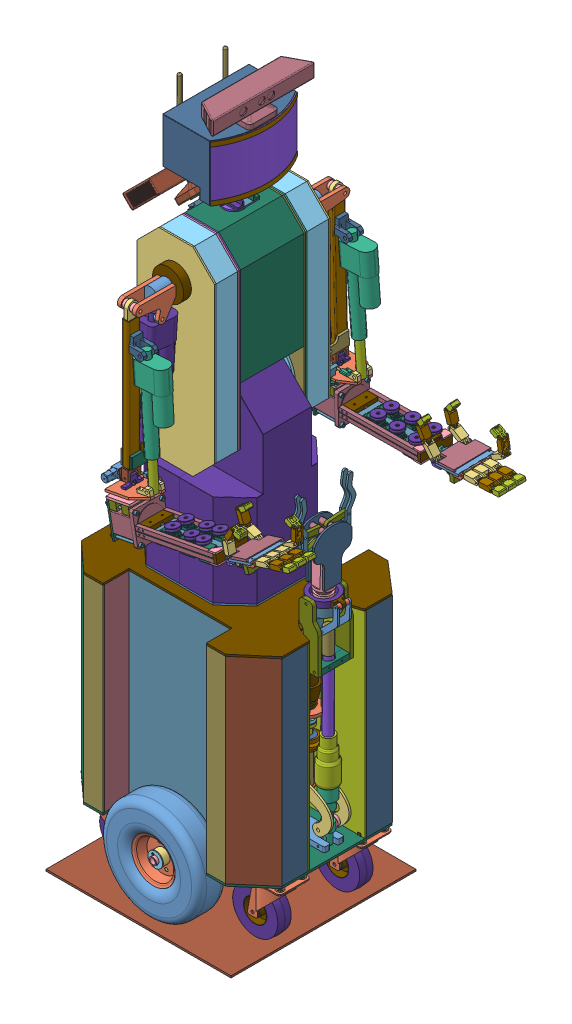
SolidWorks assembly sorbot, configuration По умолчанию. Lengths in mm. (continued)
Components (placement in the parent): (continued)
- arm.drive.p2-1: arm.drive.p2 [По умолчанию] at (43.6014 1241.2974 -35.5806) x (-0.089772 0 -0.995962) z (0.995962 0 -0.089772) size (134 5 24)
- arm.drive.p3-1: arm.drive.p3 [По умолчанию] at (3.7745 1243.7974 -50.7442) x (0 0 -1) z (0.174973 -0.984573 0) size (133.1 20 20)
- body.frame.p1-left-1: body.frame.p1-left [По умолчанию] at (-12.5682 795.4677 -226.3595) x (1 0 0) z (0 0 1) size (210 537.56 4)
- arm.drive.motor-1: arm.drive.motor [По умолчанию] at (-94.8762 1249.003 -67.2442) x (-0.533544 -0.845772 0) z (0.845772 -0.533544 0) size (117 39.5 152)
- arm.drive.motor.pair-1: arm.drive.motor.pair [По умолчанию] at (-76.8976 1162.9951 -205.8595) x (-0.885964 0.463755 0) z (0.463755 0.885964 0) size (117 39.5 152)
- arm.actuator.p2-5: arm.actuator.p2 [Default] at (-12.384 1125.8641 -368.5595) x (-0.005174 -0.093519 0.995604) z (0.999986 0 0.005196) size (20 180 20)
- arm.drive.p5-1: arm.drive.p5 [По умолчанию] at (3.7745 1243.7974 -58.7442) x (1 0 0) z (0 -1 0) size (34 8 34)
- arm.drive.p6-1: arm.drive.p6 [По умолчанию] at (3.7745 1243.7974 -50.7442) x (1 0 0) z (0 1 0) size (40 12 40)
- arm.drive.p3-2: arm.drive.p3 [По умолчанию] at (-20.8275 1162.0905 -222.3595) x (0 0 1) z (-0.923728 -0.383049 0) size (133.1 20 20)
- arm.drive.p5-2: arm.drive.p5 [По умолчанию] at (-20.8275 1162.0905 -214.3595) x (1 0 0) z (0 1 0) size (34 8 34)
- arm.drive.p6-2: arm.drive.p6 [По умолчанию] at (-20.8275 1162.0905 -222.3595) x (1 0.000029 0) z (0.000029 -1 0) size (40 12 40)
- arm.drive.p2-pair-1: arm.drive.p2-pair [По умолчанию] at (50.3811 1159.5904 -236.7848) x (-0.315418 0 0.948953) z (-0.948953 0 -0.315418) size (144 5 24)
- m14.nut-1: m14.nut [По умолчанию] at (-20.8275 1162.0905 -118.4852) x (0.513607 -0.858026 0) z (0.858026 0.513607 0) size (25.4 10.5 22.2)
- arm.drive.p7-2: arm.drive.p7 [По умолчанию] at (-14.5918 1147.0905 -123.4852) x (0 0 1) z (-1 0 0) size (28 15 59.47)
- arm.drive.p7-3: arm.drive.p7 [По умолчанию] at (-14.5918 1177.0905 -123.4852) x (0 0 -1) z (-1 0 0) size (28 15 59.47)
- arm.drive.p7-4: arm.drive.p7 [По умолчанию] at (10.1478 1228.9206 -145.3) x (0 0 1) z (-1 0 0) size (28 15 59.47)
- arm.drive.p7-5: arm.drive.p7 [По умолчанию] at (10.1478 1258.9206 -145.3) x (0 0 -1) z (-1 0 0) size (28 15 59.47)
- m14.nut-2: m14.nut [По умолчанию] at (3.7745 1243.7974 -150.3) x (-0.999875 0.015784 0) z (0.015784 0.999875 0) size (25.4 10.5 22.2)
- arm.drive.p1.m1-1: arm.drive.p1.m1 [По умолчанию] at (28.6519 1164.5905 -225.3595) x (0 1 0) z (-1 0 0) size (10 12 40)
- arm.drive.p1.m1-2: arm.drive.p1.m1 [По умолчанию] at (28.6519 1149.5905 -225.3595) x (0 1 0) z (-1 0 0) size (10 12 40)
- body.frame.p4.external-1: body.frame.p4.external [По умолчанию] at (-12.7111 795.3889 -292.3595) x (1 -0.000113 0) z (0 0 1) size (210 537.56 4)
- body.frame.p4.external-2: body.frame.p4.external [По умолчанию] at (-12.8242 795.3889 15.2558) x (1 -0.000113 0) z (0 0 1) size (210 537.56 4)
- arm.drive.p1.m1-3: arm.drive.p1.m1 [По умолчанию] at (65.4163 1231.2974 -47.7442) x (0 1 0) z (1 0 0) size (10 12 40)
- arm.drive.p1.m1-4: arm.drive.p1.m1 [По умолчанию] at (65.4163 1246.2974 -47.7442) x (0 1 0) z (1 0 0) size (10 12 40)
- body.frame.p4.right-1: body.frame.p4.right [По умолчанию] at (-12.4903 795.5195 -46.7442) x (1 0 0) z (0 0 1) size (210 537.56 4)
- arm.drive.p8-1: arm.drive.p8 [По умолчанию] at (-20.8275 1162.0905 -72.7442) x (-0.999995 0.003205 0) z (-0.003205 -0.999995 0) size (24 35.5 24)
- arm.drive.p8-2: arm.drive.p8 [По умолчанию] at (3.7745 1243.7974 -200.3595) x (1 0 0) z (0 -1 0) size (24 35.5 24)
- man1.drive1-1: man1.drive1 [По умолчанию] at (-119.3768 640.728 -141.6211) x (0.999934 0 -0.01146) z (0 1 0) size (50 50 148.25)
- body.tilit.planetary.drive.fixture.p1-1: body.tilit.planetary.drive.fixture.p1 [По умолчанию] at (-119.3768 612.7934 -141.6211) size (85 10 85)
- body.tilit.planetary.drive.fixture.p2-1: body.tilit.planetary.drive.fixture.p2 [По умолчанию] at (-119.3768 622.7934 -141.6211) size (85 4 85)
- tilt.thread.rod.fixture.2-2: tilt.thread.rod.fixture.2 [По умолчанию] at (-119.3768 793.5591 -141.6211) x (-0.837169 0 -0.546944) z (-0.546944 0 0.837169) size (40 26 40)
- body.tilit.planetary.drive.fixture.p3-1: body.tilit.planetary.drive.fixture.p3 [По умолчанию] at (-119.3768 695.728 -141.6211) size (68 8 68)
- body.tilit.planetary.drive.fixture.p4-1: body.tilit.planetary.drive.fixture.p4 [По умолчанию] at (-119.3768 753.9526 -141.6211) x (0.997546 0 -0.070011) z (0.070011 0 0.997546) size (70 9 70)
- body.tilit.planetary.drive.fixture.p5-1: body.tilit.planetary.drive.fixture.p5 [По умолчанию] at (-148.8664 612.7934 -141.6211) size (5 157 5)
- m6.nut-13: m6.nut [По умолчанию] at (-148.8664 613.2934 -141.6211) size (10 5.5 11.55)
- body.tilit.planetary.drive.fixture.p5-2: body.tilit.planetary.drive.fixture.p5 [По умолчанию] at (-89.8872 612.7934 -141.6211) size (5 157 5)
- body.tilit.planetary.drive.fixture.p5-3: body.tilit.planetary.drive.fixture.p5 [По умолчанию] at (-119.3768 612.7934 -112.1315) size (5 157 5)
- body.tilit.planetary.drive.fixture.p5-4: body.tilit.planetary.drive.fixture.p5 [По умолчанию] at (-119.3768 612.7934 -171.1107) size (5 157 5)
- m6.nut-14: m6.nut [По умолчанию] at (-89.8872 613.2934 -141.6211) size (10 5.5 11.55)
- m6.nut-15: m6.nut [По умолчанию] at (-119.3768 613.2934 -171.1107) x (0.598875 0 -0.800843) z (0.800843 0 0.598875) size (10 5.5 11.55)
- m6.nut-16: m6.nut [По умолчанию] at (-119.3768 613.2934 -112.1315) x (-0.286054 0 -0.958214) z (0.958214 0 -0.286054) size (10 5.5 11.55)
- m6.nut-17: m6.nut [По умолчанию] at (-119.3768 768.4526 -112.1315) x (-0.837169 0 -0.546944) z (-0.546944 0 0.837169) size (10 5.5 11.55)
- m6.nut-18: m6.nut [По умолчанию] at (-89.8872 768.4526 -141.6211) x (-0.837169 0 -0.546944) z (-0.546944 0 0.837169) size (10 5.5 11.55)
- m6.nut-19: m6.nut [По умолчанию] at (-119.3768 768.4526 -171.1107) x (-0.837169 0 -0.546944) z (-0.546944 0 0.837169) size (10 5.5 11.55)
- m6.nut-20: m6.nut [По умолчанию] at (-148.8664 768.4526 -141.6211) x (-0.837169 0 -0.546944) z (-0.546944 0 0.837169) size (10 5.5 11.55)
- m6.nut-21: m6.nut [По умолчанию] at (-29.5996 1324.99 9.9014) x (-0.526603 0.850111 0) z (0 0 1) size (10 5.5 11.55)
- m6.6.50mm-1: m6.6.50mm [По умолчанию] at (4.3029 1345.9909 9.9014) x (0.525089 -0.847668 0.075763) z (-0.039897 0.064407 0.997126) size (10 56 10)
- m4.nut-1: m4.nut [По умолчанию] at (-35.3987 1340.8364 4.6679) x (1 0 0) z (0 -1 0) size (6.86 5 7.92)
- m4.nut-2: m4.nut [По умолчанию] at (-103.2224 997.8992 -35.7442) x (1 0 0) z (0 -1 0) size (6.86 5 7.92)
- arm.rotate-1: arm.rotate [По умолчанию] at (22.4782 854.2475 144.4763) x (0 0 1) z (-0.185706 0.982605 0) size (85.26 111.5 91.5)
  - SY85STH65-2808A-1: SY85STH65-2808A [По умолчанию] at (-4.2017 8.56 0) size (85.26 96.5 85)
  - m6.6.80mm-1: m6.6.80mm [По умолчанию] at (-39.0017 18.56 -34.8) size (10 86 10)
  - m6.6.80mm-2: m6.6.80mm [По умолчанию] at (30.5983 18.56 34.8) size (10 86 10)
  - m6.6.80mm-3: m6.6.80mm [По умолчанию] at (30.5983 18.56 -34.8) size (10 86 10)
  - m6.6.80mm-4: m6.6.80mm [По умолчанию] at (-39.0017 18.56 34.8) size (10 86 10)
  - arm.rotate.p2-2: arm.rotate.p2 [По умолчанию] at (-46.7017 -46.44 42.5) x (1 0 0) z (0 -1 0) size (85 91.5 5)
  - m6.nut-1: m6.nut [По умолчанию] at (30.5983 -56.94 34.8) size (10 5.5 11.55)
  - m6.nut-2: m6.nut [По умолчанию] at (-39.0017 -56.94 -34.8) size (10 5.5 11.55)
  - m6.nut-3: m6.nut [По умолчанию] at (-39.0017 -56.94 34.8) size (10 5.5 11.55)
  - m6.nut-4: m6.nut [По умолчанию] at (30.5983 -56.94 -34.8) size (10 5.5 11.55)
  - arm.rotate.p1-2: arm.rotate.p1 [По умолчанию] at (-4.2017 8.56 38) x (1 0 0) z (0 -1 0) size (85 21 20)
  - arm.rotate.p1-3: arm.rotate.p1 [По умолчанию] at (-4.2017 -26.44 38) x (1 0 0) z (0 -1 0) size (85 21 20)
- arm.rotate.p8-1: arm.rotate.p8 [По умолчанию] at (-48.9081 912.5039 130.5417) x (-0.185706 0.982605 0) z (0 0 1) size (25 12 48)
- arm.rotate.p9-1: arm.rotate.p9 [По умолчанию] at (42.4949 859.0482 172.7746) x (0.982605 0.185706 0) z (0 0 1) size (30 10 65)
- arm.rotate.p9-2: arm.rotate.p9 [По умолчанию] at (72.3444 862.6542 172.7746) x (-0.982605 -0.185706 0) z (0 0 1) size (30 10 65)
- arm.elbow.rotate.p1-1: arm.elbow.rotate.p1 [По умолчанию] at (-55.7977 924.3811 168.7746) x (-0.185706 0.982605 0) z (0 0 -1) size (21.9 27.89 71.5)
- arm.rotate.p6-1: arm.rotate.p6 [По умолчанию] at (20.223 919.4631 140.2746) x (0 0 1) z (-0.982605 -0.185706 0) size (85 6 102)
- arm.rotate.p7-1: arm.rotate.p7 [По умолчанию] at (81.3033 937.1131 170.2746) x (-0.185706 0.982605 0) z (0 0 -1) size (16 36 10)
- arm.rotate.p7-2: arm.rotate.p7 [По умолчанию] at (81.3033 937.1131 140.2746) x (-0.185706 0.982605 0) z (0 0 -1) size (16 36 10)
- arm.rotate.p10-1: arm.rotate.p10 [По умолчанию] at (-37.1666 892.8424 182.7746) x (0 0 -1) z (0.982605 0.185706 0) size (85 6 65)
- arm.elbow.rotate.bearing-1: arm.elbow.rotate.bearing [По умолчанию] at (-7.5173 911.1932 140.056) x (-0.183128 -0.03461 0.98248) z (-0.96539 -0.182453 -0.18637) size (61.4 10 61.4)
  - arm.elbow.rotate.bearing.p1-1: arm.elbow.rotate.bearing.p1 [По умолчанию] at (0.2225 -3.7755 0) size (61.4 4.5 61.4)
  - ball.10mm-1: ball.10mm [По умолчанию] at (0.0947 -1.5255 -24.7664) size (10 10 10)
  - ball.10mm-2: ball.10mm [По умолчанию] at (-9.9677 -1.5255 -22.5733) x (0.913545 0 -0.406737) z (0.406737 0 0.913545) size (10 10 10)
  - ball.10mm-3: ball.10mm [По умолчанию] at (-18.2681 -1.5255 -16.477) x (0.669131 0 -0.743145) z (0.743145 0 0.669131) size (10 10 10)
  - ball.10mm-4: ball.10mm [По умолчанию] at (-23.3713 -1.5255 -7.5317) x (0.309017 0 -0.951057) z (0.951057 0 0.309017) size (10 10 10)
  - ball.10mm-5: ball.10mm [По умолчанию] at (-24.3949 -1.5255 2.7159) x (-0.104528 0 -0.994522) z (0.994522 0 -0.104528) size (10 10 10)
  - ball.10mm-6: ball.10mm [По умолчанию] at (-21.162 -1.5255 12.4939) x (-0.5 0 -0.866025) z (0.866025 0 -0.5) size (10 10 10)
  - ball.10mm-7: ball.10mm [По умолчанию] at (-14.2315 -1.5255 20.1116) x (-0.809017 0 -0.587785) z (0.587785 0 -0.809017) size (10 10 10)
  - ball.10mm-8: ball.10mm [По умолчанию] at (-4.8018 -1.5255 24.2518) x (-0.978148 0 -0.207912) z (0.207912 0 -0.978148) size (10 10 10)
  - ball.10mm-9: ball.10mm [По умолчанию] at (5.4967 -1.5255 24.1987) x (-0.978148 0 0.207912) z (-0.207912 0 -0.978148) size (10 10 10)
  - ball.10mm-10: ball.10mm [По умолчанию] at (14.8832 -1.5255 19.9614) x (-0.809017 0 0.587785) z (-0.587785 0 -0.809017) size (10 10 10)
  - ball.10mm-11: ball.10mm [По умолчанию] at (21.7347 -1.5255 12.2726) x (-0.5 0 0.866025) z (-0.866025 0 -0.5) size (10 10 10)
  - ball.10mm-12: ball.10mm [По умолчанию] at (24.8666 -1.5255 2.4617) x (-0.104528 0 0.994522) z (-0.994522 0 -0.104528) size (10 10 10)
  - ball.10mm-13: ball.10mm [По умолчанию] at (23.7373 -1.5255 -7.7748) x (0.309017 0 0.951057) z (-0.951057 0 0.309017) size (10 10 10)
  - ball.10mm-14: ball.10mm [По умолчанию] at (18.542 -1.5255 -16.6669) x (0.669131 0 0.743145) z (-0.743145 0 0.669131) size (10 10 10)
  - ball.10mm-15: ball.10mm [По умолчанию] at (10.1792 -1.5255 -22.6772) x (0.913545 0 0.406737) z (-0.406737 0 0.913545) size (10 10 10)
- arm.elbow.rotate.p3-1: arm.elbow.rotate.p3 [По умолчанию] at (-6.3462 904.7735 140.2746) x (0.982605 0.185706 0) z (0 0 1) size (36.4 9 36.4)
- arm.elbow.rotate.p4-1: arm.elbow.rotate.p4 [По умолчанию] at (-6.3462 904.7735 140.2746) x (0.982605 0.185706 0) z (0 0 1) size (22 7 22)
- bolt.m8.short-1: bolt.m8.short [По умолчанию] at (-3.7463 891.017 140.2746) x (0.982605 0.185706 0) z (0 0 1) size (12.8 43 12.8)
- m8.nut-1: m8.nut [По умолчанию] at (-9.2247 920.0039 140.2746) x (0.979774 0.185171 -0.075859) z (0.07454 0.014088 0.997119) size (14.97 7 13.53)
- arm.rotate.p11-1: arm.rotate.p11 [По умолчанию] at (-41.1593 913.9684 141.7746) x (-0.185706 0.982605 0) z (0 0 -1) size (24 14 44)
- arm.elbow.rotate.p5-1: arm.elbow.rotate.p5 [По умолчанию] at (-37.816 927.7795 114.7746) x (-0.0817 0.432291 -0.898025) z (0.982605 0.185706 0) size (5 5 75)
- arm.elbow.rotate.p6-1: arm.elbow.rotate.p6 [По умолчанию] at (39.7316 938.238 120.2746) x (0 0 1) z (-0.982685 -0.185282 0) size (21 8 17.99)
- arm.elbow.rotate.p11-1: arm.elbow.rotate.p11 [По умолчанию] at (-1.3122 934.6785 114.7746) x (0 0 -1) z (0.982605 0.185706 0) size (29.5 27.93 10)
- arm.elbow.rotate.p12-1: arm.elbow.rotate.p12 [По умолчанию] at (0.0407 905.9806 81.7746) x (0.589563 0.111424 0.8) z (-0.786084 -0.148565 0.6) size (29 4.5 14)
- arm.elbow.rotate.p13-1: arm.elbow.rotate.p13 [По умолчанию] at (-28.3338 929.5716 114.7746) x (-0.185706 0.982605 0) z (0 0 1) size (9 12 9)
- arm.elbow.rotate.p14-1: arm.elbow.rotate.p14 [По умолчанию] at (-41.599 927.0645 114.7746) x (0 0 -1) z (0.982605 0.185706 0) size (18 18 10)
- palm.tilt.p1-1: palm.tilt.p1 [По умолчанию] at (76.6621 839.8086 140.4246) x (0.185706 -0.982605 0) z (0 0 1) size (36.5 37.1 24.8)
- palm.drives.fixture-2: palm.drives.fixture [По умолчанию] at (72.6077 850.4915 150.4246) x (0.982605 0.185706 0) z (0 0 -1) size (30.05 15 65)
- palm.lift.p2-2: palm.lift.p2 [По умолчанию] at (97.1945 857.1737 140.4246) x (0.033136 -0.175327 -0.983952) z (0.982605 0.185706 0) size (5 5 158)
- palm.drive.thread.fixture.p2-1: palm.drive.thread.fixture.p2 [По умолчанию] at (87.8616 855.4098 140.4246) x (-0.05957 0.315194 0.947156) z (0.982605 0.185706 0) size (11.8 11.8 25)
- m3x8-1: m3x8 [По умолчанию] at (92.8919 850.6734 142.3172) x (0.982605 0.185707 0) z (0.05957 -0.315194 -0.947156) size (5.3 6.85 5.3)
- m3x8-2: m3x8 [По умолчанию] at (101.0372 852.2128 142.3172) x (0.982605 0.185707 0) z (0.05957 -0.315194 -0.947156) size (5.3 6.85 5.3)
- palm.drive.thread.fixture-1: palm.drive.thread.fixture [По умолчанию] at (254.7288 885.7804 140.4246) x (0 0 -1) z (-0.982605 -0.185706 0) size (30 34 7)
- palm.lift.fixture-1: palm.lift.fixture [По умолчанию] at (260.6332 900.2751 126.1211) x (0 0 -1) z (0.185706 -0.982605 0) size (30 17 12)
- palm.lift.fixture.p2-1: palm.lift.fixture.p2 [По умолчанию] at (287.8736 901.2786 140.2746) x (0 0 1) z (-0.950223 -0.311571 0) size (26 12.5 30)
- PALM.LIFT.THREAD.FIXTURE.P3-1: PALM.LIFT.THREAD.FIXTURE.P3 [По умолчанию] at (131.0658 873.7522 140.2958) x (-0.982605 -0.185706 0) z (0 0 1) size (20 14 10)
- palm.lift.drive.nut-1: palm.lift.drive.nut [По умолчанию] at (168.1531 870.5844 140.4246) x (0.124167 -0.656989 -0.743604) z (0.982605 0.185706 0) size (12 12 16)
- palm.lift.nut.fixture-1: palm.lift.nut.fixture [По умолчанию] at (174.1569 881.8961 145.4246) x (0 0 -1) z (-0.982605 -0.185706 0) size (10 28 10)
- palm.lift.nut.fixture-2: palm.lift.nut.fixture [По умолчанию] at (174.1569 881.8961 135.4246) x (0 0 1) z (0.982605 0.185706 0) size (10 28 10)
- palm.lift.p4-1: palm.lift.p4 [По умолчанию] at (168.591 857.4974 140.4246) x (0 0 -1) z (0.982605 0.185706 0) size (4 4 120)
- palm.lift.fixture.p6-1: palm.lift.fixture.p6 [По умолчанию] at (276.6776 877.9252 140.4246) x (0 0 -1) z (0.982605 0.185706 0) size (12 12 20.44)
- palm.lift.fixture.p7-1: palm.lift.fixture.p7 [По умолчанию] at (292.1321 880.846 138.4246) x (0.730069 0.683374 0) z (0 0 1) size (27 9 4)
- m6.washer-1: m6.washer [По умолчанию] at (284.4317 914.5677 140.506) x (0.950223 0.311571 0.000222) z (-0.000211 -0.000069 1) size (18 1.7 18)
- m6.washer-2: m6.washer [По умолчанию] at (289.4791 899.1741 140.506) x (-0.950223 -0.311571 -0.000219) z (-0.000208 -0.000068 1) size (18 1.7 18)
- m6.washer-3: m6.washer [По умолчанию] at (286.8308 907.251 140.506) x (0.950223 0.311571 0.000222) z (-0.000211 -0.000069 1) size (18 1.7 18)
- palm.lift.on-palm.fixture-2: palm.lift.on-palm.fixture [По умолчанию] at (300.1799 895.8423 140.2746) x (0 0 -1) z (0.950223 0.311571 0) size (26 23.89 8)
- palm.lift.p1-1: palm.lift.p1 [По умолчанию] at (338.412 919.9816 174.4917) x (0.950144 0.311545 0.012888) z (-0.311571 0.950223 0) size (36.5 37.1 24.8)
- palm.drive.thread.fixture.p2-2: palm.drive.thread.fixture.p2 [По умолчанию] at (325.9934 915.9097 160.372) x (-0.999321 0.034794 -0.0121) z (0.012247 0.004016 -0.999917) size (11.8 11.8 25)
- palm.tilit.fixture-1: palm.tilit.fixture [По умолчанию] at (336.6565 929.587 176.5089) x (0.012247 0.004016 -0.999917) z (-0.950144 -0.311545 -0.012888) size (12 17 18)
- palm.tilit.p8-1: palm.tilit.p8 [По умолчанию] at (326.1771 915.9699 145.3733) x (-0.999829 0.013918 -0.01219) z (0.012247 0.004016 -0.999917) size (5 5 57)
- palm.tilit.p9-1: palm.tilit.p9 [По умолчанию] at (336.3842 931.6025 91.2066) x (-0.950144 -0.311545 -0.012888) z (-0.012247 -0.004016 0.999917) size (23.81 15.6 6)
- palm.tilit.p10-1: palm.tilit.p10 [По умолчанию] at (303.1082 912.5882 153.2746) x (0 0 -1) z (0.950223 0.311571 0) size (26 8.5 15)
- palm.tilit.p11-1: palm.tilit.p11 [По умолчанию] at (326.5434 916.09 115.4643) x (0.950144 0.311545 0.012888) z (-0.012247 -0.004016 0.999917) size (17.95 8 10)
- palm.tilit.p12-1: palm.tilit.p12 [По умолчанию] at (317.7933 904.2485 140.2746) x (0.070018 0.022958 -0.997282) z (0.94764 0.310724 0.073685) size (29 4 9)
- arm.rotate.p6-2: arm.rotate.p6 [По умолчанию] at (17.2833 914.2431 -421.887) x (-0.005195 -0.022106 0.999742) z (-0.99991 -0.012267 -0.005467) size (85 6 102)
- arm.rotate.p8-2: arm.rotate.p8 [По умолчанию] at (-52.6122 919.605 -432.1343) x (-0.012385 0.99968 0.022041) z (-0.005195 -0.022106 0.999742) size (25 12 48)
- arm.rotate.p7-3: arm.rotate.p7 [По умолчанию] at (80.4988 921.0176 -421.4088) x (-0.012385 0.99968 0.022041) z (0.005195 0.022106 -0.999742) size (16 36 10)
- arm.rotate.p7-4: arm.rotate.p7 [По умолчанию] at (80.343 920.3544 -391.4165) x (-0.012385 0.99968 0.022041) z (0.005195 0.022106 -0.999742) size (16 36 10)
- bolt.m8.short-2: bolt.m8.short [По умолчанию] at (-11.2814 892.2812 -422.5211) x (0.999923 0.012406 -0.000807) z (0.00108 -0.022029 0.999757) size (12.8 43 12.8)
- m8.nut-2: m8.nut [По умолчанию] at (-11.6234 919.8874 -421.9124) x (0.559915 -0.011329 0.828472) z (-0.828457 -0.022602 0.559596) size (14.97 7 13.53)
- arm.elbow.rotate.bearing-2: arm.elbow.rotate.bearing [По умолчанию] at (-11.6907 910.4164 -422.2454) x (0.829913 -0.002018 0.557889) z (-0.557755 -0.025201 0.829623) size (61.4 10 61.4)
  - arm.elbow.rotate.bearing.p1-1: arm.elbow.rotate.bearing.p1 [По умолчанию] at (0.2225 -3.7755 0) size (61.4 4.5 61.4)
  - ball.10mm-1: ball.10mm [По умолчанию] at (0.0947 -1.5255 -24.7664) size (10 10 10)
  - ball.10mm-2: ball.10mm [По умолчанию] at (-9.9677 -1.5255 -22.5733) x (0.913545 0 -0.406737) z (0.406737 0 0.913545) size (10 10 10)
  - ball.10mm-3: ball.10mm [По умолчанию] at (-18.2681 -1.5255 -16.477) x (0.669131 0 -0.743145) z (0.743145 0 0.669131) size (10 10 10)
  - ball.10mm-4: ball.10mm [По умолчанию] at (-23.3713 -1.5255 -7.5317) x (0.309017 0 -0.951057) z (0.951057 0 0.309017) size (10 10 10)
  - ball.10mm-5: ball.10mm [По умолчанию] at (-24.3949 -1.5255 2.7159) x (-0.104528 0 -0.994522) z (0.994522 0 -0.104528) size (10 10 10)
  - ball.10mm-6: ball.10mm [По умолчанию] at (-21.162 -1.5255 12.4939) x (-0.5 0 -0.866025) z (0.866025 0 -0.5) size (10 10 10)
  - ball.10mm-7: ball.10mm [По умолчанию] at (-14.2315 -1.5255 20.1116) x (-0.809017 0 -0.587785) z (0.587785 0 -0.809017) size (10 10 10)
  - ball.10mm-8: ball.10mm [По умолчанию] at (-4.8018 -1.5255 24.2518) x (-0.978148 0 -0.207912) z (0.207912 0 -0.978148) size (10 10 10)
  - ball.10mm-9: ball.10mm [По умолчанию] at (5.4967 -1.5255 24.1987) x (-0.978148 0 0.207912) z (-0.207912 0 -0.978148) size (10 10 10)
  - ball.10mm-10: ball.10mm [По умолчанию] at (14.8832 -1.5255 19.9614) x (-0.809017 0 0.587785) z (-0.587785 0 -0.809017) size (10 10 10)
  - ball.10mm-11: ball.10mm [По умолчанию] at (21.7347 -1.5255 12.2726) x (-0.5 0 0.866025) z (-0.866025 0 -0.5) size (10 10 10)
  - ball.10mm-12: ball.10mm [По умолчанию] at (24.8666 -1.5255 2.4617) x (-0.104528 0 0.994522) z (-0.994522 0 -0.104528) size (10 10 10)
  - ball.10mm-13: ball.10mm [По умолчанию] at (23.7373 -1.5255 -7.7748) x (0.309017 0 0.951057) z (-0.951057 0 0.309017) size (10 10 10)
  - ball.10mm-14: ball.10mm [По умолчанию] at (18.542 -1.5255 -16.6669) x (0.669131 0 0.743145) z (-0.743145 0 0.669131) size (10 10 10)
  - ball.10mm-15: ball.10mm [По умолчанию] at (10.1792 -1.5255 -22.6772) x (0.913545 0 0.406737) z (-0.406737 0 0.913545) size (10 10 10)
- arm.elbow.rotate.p4-2: arm.elbow.rotate.p4 [По умолчанию] at (-11.4253 903.8925 -422.2651) x (0.756023 0.023788 -0.654112) z (0.654428 -0.008562 0.756076) size (22 7 22)
- arm.elbow.rotate.p3-2: arm.elbow.rotate.p3 [По умолчанию] at (-11.4253 903.8925 -422.2651) x (0.999923 0.012396 -0.000381) z (0.000654 -0.022034 0.999757) size (36.4 9 36.4)
- arm.rotate.p10-2: arm.rotate.p10 [По умолчанию] at (-43.7015 904.4334 -464.9318) x (-0.005195 -0.022106 0.999742) z (0.99991 0.012267 0.005467) size (85 6 65)
- arm.rotate-2: arm.rotate [По умолчанию] at (8.1724 849.0496 -419.1732) x (-0.005195 -0.022106 0.999742) z (-0.012385 0.99968 0.022041) size (85.26 111.5 91.5)
  - SY85STH65-2808A-1: SY85STH65-2808A [По умолчанию] at (-4.2017 8.56 0) size (85.26 96.5 85)
  - m6.6.80mm-1: m6.6.80mm [По умолчанию] at (-39.0017 18.56 -34.8) size (10 86 10)
  - m6.6.80mm-2: m6.6.80mm [По умолчанию] at (30.5983 18.56 34.8) size (10 86 10)
  - m6.6.80mm-3: m6.6.80mm [По умолчанию] at (30.5983 18.56 -34.8) size (10 86 10)
  - m6.6.80mm-4: m6.6.80mm [По умолчанию] at (-39.0017 18.56 34.8) size (10 86 10)
  - arm.rotate.p2-2: arm.rotate.p2 [По умолчанию] at (-46.7017 -46.44 42.5) x (1 0 0) z (0 -1 0) size (85 91.5 5)
  - m6.nut-1: m6.nut [По умолчанию] at (30.5983 -56.94 34.8) size (10 5.5 11.55)
  - m6.nut-2: m6.nut [По умолчанию] at (-39.0017 -56.94 -34.8) size (10 5.5 11.55)
  - m6.nut-3: m6.nut [По умолчанию] at (-39.0017 -56.94 34.8) size (10 5.5 11.55)
  - m6.nut-4: m6.nut [По умолчанию] at (30.5983 -56.94 -34.8) size (10 5.5 11.55)
  - arm.rotate.p1-2: arm.rotate.p1 [По умолчанию] at (-4.2017 8.56 38) x (1 0 0) z (0 -1 0) size (85 21 20)
  - arm.rotate.p1-3: arm.rotate.p1 [По умолчанию] at (-4.2017 -26.44 38) x (1 0 0) z (0 -1 0) size (85 21 20)
- arm.rotate.p9-3: arm.rotate.p9 [По умолчанию] at (59.0931 848.0507 -390.6251) x (-0.99991 -0.012267 -0.005467) z (-0.005195 -0.022106 0.999742) size (30 10 65)
- arm.rotate.p9-4: arm.rotate.p9 [По умолчанию] at (29.0711 849.682 -390.745) x (0.99991 0.012267 0.005467) z (-0.005195 -0.022106 0.999742) size (30 10 65)
- arm.rotate.p11.mirr-1: arm.rotate.p11.mirr [По умолчанию] at (-44.3413 918.5492 -379.6011) x (-0.012385 0.99968 0.022041) z (0.005195 0.022106 -0.999742) size (24 14 44)
- arm.elbow.rotate.p1-2: arm.elbow.rotate.p1 [По умолчанию] at (-56.5709 932.0381 -450.3776) x (0.012299 -0.999907 -0.005858) z (-0.005395 -0.005924 0.999968) size (21.9 27.89 71.5)
- arm.elbow.rotate.p6.mirr-1: arm.elbow.rotate.p6.mirr [По умолчанию] at (20.3416 928.6659 -401.5471) x (0.005195 0.022106 -0.999742) z (0.99991 0.012267 0.005467) size (21 8 17.99)
- arm.elbow.rotate.p13-2: arm.elbow.rotate.p13 [По умолчанию] at (-28.5648 932.0653 -396.2246) x (0.012299 -0.999907 -0.005858) z (0.005395 0.005924 -0.999968) size (9 12 9)
- arm.elbow.rotate.p14-2: arm.elbow.rotate.p14 [По умолчанию] at (-42.4135 931.8954 -396.3003) x (0.005872 -0.033224 -0.999431) z (0.99991 0.012267 0.005467) size (18 18 10)
- arm.elbow.rotate.p5-2: arm.elbow.rotate.p5 [По умолчанию] at (-38.5639 931.9427 -396.2793) x (0.005872 -0.033224 -0.999431) z (0.99991 0.012267 0.005467) size (5 5 75)
- arm.elbow.rotate.p11-2: arm.elbow.rotate.p11 [По умолчанию] at (8.5819 932.5211 -396.0215) x (-0.005195 -0.022106 0.999742) z (-0.99991 -0.012267 -0.005467) size (29.5 27.93 10)
- arm.elbow.rotate.p12-2: arm.elbow.rotate.p12 [По умолчанию] at (-5.2424 903.6993 -363.7222) x (0.604102 0.025046 -0.796513) z (0.796811 -0.00345 0.604219) size (29 4.5 14)
- palm.drives.fixture-3: palm.drives.fixture [По умолчанию] at (57.358 836.5241 -413.2447) x (0.99991 0.012267 0.005467) z (0.005195 0.022106 -0.999742) size (30.05 15 65)
- palm.tilt.p1-2: palm.tilt.p1 [По умолчанию] at (59.5491 825.5233 -423.4792) x (0.012385 -0.99968 -0.022041) z (-0.005195 -0.022106 0.999742) size (36.5 37.1 24.8)
- palm.drive.thread.fixture.p2-3: palm.drive.thread.fixture.p2 [По умолчанию] at (73.3338 838.9402 -423.1109) x (0.002801 0.207624 -0.978205) z (0.99991 0.012267 0.005467) size (11.8 11.8 25)
- palm.lift.p2-3: palm.lift.p2 [По умолчанию] at (85.2879 839.0868 -423.0455) x (0.006111 -0.053098 -0.998571) z (0.99991 0.012267 0.005467) size (5 5 158)
- palm.lift.drive.nut-2: palm.lift.drive.nut [По умолчанию] at (152.3766 839.9099 -422.6787) x (-0.003006 -0.192356 0.981321) z (0.99991 0.012267 0.005467) size (12 12 16)
- palm.lift.nut.fixture-3: palm.lift.nut.fixture [По умолчанию] at (160.2261 849.8943 -417.4158) x (0.005195 0.022106 -0.999742) z (-0.99991 -0.012267 -0.005467) size (10 28 10)
- palm.lift.nut.fixture-4: palm.lift.nut.fixture [По умолчанию] at (160.278 850.1154 -427.4132) x (-0.005195 -0.022106 0.999742) z (0.99991 0.012267 0.005467) size (10 28 10)
- palm.lift.p4-2: palm.lift.p4 [По умолчанию] at (150.9783 826.9543 -422.9724) x (-0.009526 0.934752 -0.355174) z (0.99991 0.012267 0.005467) size (4 4 120)
- palm.lift.fixture-2: palm.lift.fixture [По умолчанию] at (251.2934 853.4367 -436.1728) x (0.005195 0.022106 -0.999742) z (0.012385 -0.99968 -0.022041) size (30 17 12)
- palm.lift.fixture.p2-2: palm.lift.fixture.p2 [По умолчанию] at (278.3444 848.1669 -421.9915) x (-0.005195 -0.022106 0.999742) z (-0.998179 -0.059975 -0.006513) size (26 12.5 30)
- palm.drive.thread.fixture-2: palm.drive.thread.fixture [По умолчанию] at (243.3826 839.8806 -422.2064) x (0.005195 0.022106 -0.999742) z (-0.99991 -0.012267 -0.005467) size (30 34 7)
- m6.washer-4: m6.washer [По умолчанию] at (279.3618 845.7191 -421.8089) x (-0.988782 -0.062508 0.135656) z (0.136738 -0.013357 0.990517) size (18 1.7 18)
- m6.washer-5: m6.washer [По умолчанию] at (278.8509 854.2017 -421.624) x (-0.923349 -0.063864 0.378614) z (-0.379229 -0.002669 -0.925299) size (18 1.7 18)
- m6.washer-6: m6.washer [По умолчанию] at (278.3881 861.886 -421.4565) x (-0.923349 -0.063864 0.378614) z (-0.379229 -0.002669 -0.925299) size (18 1.7 18)
- palm.lift.fixture.p6-2: palm.lift.fixture.p6 [По умолчанию] at (260.9684 828.3037 -422.371) x (0.005195 0.022106 -0.999742) z (0.99991 0.012267 0.005467) size (12 12 20.44)
- palm.lift.on-palm.fixture-3: palm.lift.on-palm.fixture [По умолчанию] at (288.8671 839.7851 -422.1222) x (0.005195 0.022106 -0.999742) z (0.998179 0.059975 0.006513) size (26 23.89 8)
- palm.lift.fixture.p7-2: palm.lift.fixture.p7 [По умолчанию] at (276.6855 828.4557 -420.4355) x (0.911851 0.41029 0.013811) z (0.005195 0.022106 -0.999742) size (27 9 4)
- palm.tilit.fixture-2: palm.tilit.fixture [По умолчанию] at (333.8862 862.4481 -385.8466) x (0.005195 0.022106 -0.999742) z (-0.998179 -0.059975 -0.006513) size (12 17 18)
- palm.lift.p1-2: palm.lift.p1 [По умолчанию] at (332.7336 852.6936 -388.0688) x (0.998179 0.059975 0.006513) z (-0.060104 0.997955 0.021755) size (36.5 37.1 24.8)
- palm.drive.thread.fixture.p2-4: palm.drive.thread.fixture.p2 [По умолчанию] at (319.5802 852.2073 -402.1015) x (0.991144 0.132548 0.008081) z (0.005195 0.022106 -0.999742) size (11.8 11.8 25)
- palm.tilit.p8-2: palm.tilit.p8 [По умолчанию] at (319.9542 853.799 -474.0829) x (0.998896 -0.046783 0.004156) z (-0.005195 -0.022106 0.999742) size (5 5 57)
- palm.tilit.p9-2: palm.tilit.p9 [По умолчанию] at (333.0838 866.2226 -471.0893) x (-0.998179 -0.059975 -0.006513) z (-0.005195 -0.022106 0.999742) size (23.81 15.6 6)
- palm.tilit.p10-2: palm.tilit.p10 [По умолчанию] at (295.8835 854.9468 -408.7471) x (0.005195 0.022106 -0.999742) z (0.998179 0.059975 0.006513) size (26 8.5 15)
- palm.tilit.p12-2: palm.tilit.p12 [По умолчанию] at (308.0373 843.4408 -421.9418) x (0.090521 0.027153 -0.995524) z (0.994079 0.057865 0.091968) size (29 4 9)
- palm.tilit.p11-2: palm.tilit.p11 [По умолчанию] at (319.8114 853.1912 -446.5982) x (0.998179 0.059975 0.006513) z (-0.005195 -0.022106 0.999742) size (17.95 8 10)
- SY57STH56-2804A-1: SY57STH56-2804A [Default] at (-12.4903 1378.2936 -136.5542) x (1 0 0) z (0 0 1) size (56 76.6 56)
- head.tilt.p1-1: head.tilt.p1 [По умолчанию] at (-12.4903 1438.7936 -136.5542) x (0.436164 0 -0.899867) z (0.899867 0 0.436164) size (54 17.5 54)
- head.rotate.bearing-1: head.rotate.bearing [По умолчанию] at (-12.4903 1435.8936 -136.5542) x (1 0 0) z (0 0 1) size (30 8.9 30)
- head.rotate.bearing.insert-1: head.rotate.bearing.insert [По умолчанию] at (-12.4903 1435.8936 -136.5542) x (1 0 0) z (0 0 1) size (17 8.5 17)
- SY42STH47-1: SY42STH47 [Default] at (-33.8403 1484.4436 -199.0542) x (-1 0 0) z (0 1 0) size (42.3 76 42.3)
- head.tilt.p2-1: head.tilt.p2 [По умолчанию] at (-33.8403 1484.4436 -144.3542) x (-0.997593 -0.06934 0) z (-0.06934 0.997593 0) size (15 9.8 14.97)
- head.tilit.p4-1: head.tilit.p4 [По умолчанию] at (-2.6766 1441.2936 -156.8012) x (1 0 0) z (0 0 1) size (9.2 13.5 9.2)
- head.tilit.p4-2: head.tilit.p4 [По умолчанию] at (7.7567 1441.2936 -126.7405) x (1 0 0) z (0 0 1) size (9.2 13.5 9.2)
- head.tilit.p4-3: head.tilit.p4 [По умолчанию] at (-22.304 1441.2936 -116.3072) x (1 0 0) z (0 0 1) size (9.2 13.5 9.2)
- head.tilit.p4-4: head.tilit.p4 [По умолчанию] at (-32.7373 1441.2936 -146.3679) x (1 0 0) z (0 0 1) size (9.2 13.5 9.2)
- head.p1-1: head.p1 [По умолчанию] at (-12.4903 1454.7936 -136.5542) x (0 0 -1) z (1 0 0) size (58.13 3.5 85)
- head.tilit.p5-1: head.tilit.p5 [По умолчанию] at (-54.9903 1463.2936 -152.0542) x (0 0 -1) z (1 0 0) size (16 47.3 85)
- head.tilt.p8-1: head.tilt.p8 [По умолчанию] at (-4.1768 1486.067 -139.0542) x (-0.002177 0.999998 0) z (0.999998 0.002177 0) size (45.99 8.9 45.99)
- head.tilit.p5.m-1: head.tilit.p5.m [По умолчанию] at (30.0097 1463.2936 -117.9254) x (0 0 1) z (-1 0 0) size (16 47.3 85)
- head.tilt.p10-1: head.tilt.p10 [По умолчанию] at (-4.1768 1486.067 -141.5542) x (0.999434 0.033636 0) z (0.033636 -0.999434 0) size (36 3.5 36)
- head.tilt.p10-2: head.tilt.p10 [По умолчанию] at (-4.1768 1486.067 -131.6542) x (0.999434 0.033636 0) z (-0.033636 0.999434 0) size (36 3.5 36)
- head.tilit.p11-1: head.tilit.p11 [По умолчанию] at (-4.1768 1486.067 -131.6542) x (0.999434 0.033636 0) z (0.033636 -0.999434 0) size (36 3.5 113)
- head.tilit.p11-2: head.tilit.p11 [По умолчанию] at (-4.1768 1486.067 -145.0542) x (0.999434 0.033636 0) z (0.033636 -0.999434 0) size (36 3.5 113)
- m4.nut-3: m4.nut [По умолчанию] at (4.9956 1495.2794 -123.1542) x (1 0 0) z (0 1 0) size (6.86 5 7.92)
- m4.nut-4: m4.nut [По умолчанию] at (-4.2051 1499.067 -123.1542) x (1 0 0) z (0 1 0) size (6.86 5 7.92)
- m4.nut-5: m4.nut [По умолчанию] at (5.0356 1476.8947 -123.1542) x (1 0 0) z (0 1 0) size (6.86 5 7.92)
- m4.nut-6: m4.nut [По умолчанию] at (-4.1485 1473.067 -123.1542) x (1 0 0) z (0 1 0) size (6.86 5 7.92)
- m4.nut-7: m4.nut [По умолчанию] at (-13.3492 1476.8546 -123.1542) x (1 0 0) z (0 1 0) size (6.86 5 7.92)
- head.tilt.p12-2: head.tilt.p12 [По умолчанию] at (-4.1768 1486.067 -148.0542) x (1 0 0) z (0 0 1) size (18 18 3)
- m4.nut-8: m4.nut [По умолчанию] at (-13.3892 1495.2394 -123.1542) x (1 0 0) z (0 1 0) size (6.86 5 7.92)
- head.tilt.p9-1: head.tilt.p9 [По умолчанию] at (-4.1768 1486.067 -157.7074) x (0.92329 -0.384104 0) z (0 0 1) size (6 6 45)
- m6.washer-7: m6.washer [По умолчанию] at (-4.1768 1486.067 -117.9254) x (1 0 0) z (0 -1 0) size (18 1.7 18)
- m6.washer-8: m6.washer [По умолчанию] at (-4.1768 1486.067 -152.0542) x (1 0 0) z (0 1 0) size (18 1.7 18)
- head.tilt.p12.m-1: head.tilt.p12.m [По умолчанию] at (-4.1768 1486.067 -128.1542) x (1 0 0) z (0 0 1) size (18 18 6.5)
- head.tilt.p13-1: head.tilt.p13 [По умолчанию] at (-6.8677 1566.0217 -131.6542) x (1 0 0) z (0 1 0) size (30 9.9 30) (hidden)
- head.p3-1: head.p3 [По умолчанию] at (8.1323 1551.1571 -126.1542) x (0 0 1) z (-1 0 0) size (14 31.97 30)
- head.p3-2: head.p3 [По умолчанию] at (-21.8677 1551.1571 -147.0542) x (0 0 -1) z (1 0 0) size (14 31.97 30)
- head.p2-1: head.p2 [По умолчанию] at (-6.6891 1547.1571 -136.5542) x (0 0 -1) z (1 0 0) size (154.89 2 65.43)
- logitech.sphere.af-1: logitech.sphere.af [По умолчанию] at (23.3461 1596.1571 -74.1093) x (0 0 -1) z (1 0 0) size (77.78 90.89 77.78)
- logitech.sphere.af-2: logitech.sphere.af [По умолчанию] at (23.3461 1596.1571 -198.999) x (0 0 -1) z (1 0 0) size (77.78 90.89 77.78)
- head.glass-1: head.glass [По умолчанию] at (-15.5992 1517.1571 -268.7053) x (0.000076 0 1) z (-1 0 0.000076) size (235 150 37.51)
- head.glass.fixture-1: head.glass.fixture [По умолчанию] at (76.9123 1529.1571 -118.3804) x (-0.000076 0 -1) z (0 -1 0) size (235.55 35.5 12)
- head.glass.fixture-2: head.glass.fixture [По умолчанию] at (76.9123 1667.1571 -118.3804) x (-0.000076 0 -1) z (0 -1 0) size (235.55 35.5 12)
- head.p4-1: head.p4 [По умолчанию] at (73.3132 1518.1571 -118.364) x (0 0 -1) z (0 -1 0) size (233.94 161.62 151)
- kinect-1: kinect [По умолчанию] at (-159.5074 1437.4644 -132.5396) x (0 0 -1) z (0.707107 0.707107 0) size (276 72 65)
- ant-2: ant [По умолчанию] at (-84.6104 1643.7707 -198.1028) x (0 0 1) z (-1 0 0) size (10 94.18 17)
- ant-3: ant [По умолчанию] at (-84.6104 1643.7707 -74.539) x (0 0 1) z (-1 0 0) size (10 94.18 17)
- kinect-black-1: kinect-black [По умолчанию] at (68.8437 1721.1571 -136.5839) x (0 0 1) z (-1 0 0) size (276 72 65)
- S03T STD GWS Servo-1: S03T STD GWS Servo [Default] at (-64.1673 1385.2578 -131.3796) x (0.707107 0.707107 0) z (0 0 1) size (20.32 45.88 53.29)
- back-kinect-servo-1: back-kinect-servo [По умолчанию] at (-97.4588 1418.5493 -132.5396) x (0.707107 0.707107 0) z (0 0 1) size (44.5 5.25 44.5)
- back-kinect-fixture-1: back-kinect-fixture [По умолчанию] at (-120.6166 1398.5735 -132.5396) x (0 0 -1) z (0.707107 0.707107 0) size (80 2 65)
- body.cover-1: body.cover [По умолчанию] at (14.9352 1082.7934 -136.9555) x (0 0 -1) z (1 0 0) size (278.72 470.5 152.62)
- body.cover-2: body.cover [По умолчанию] at (-55.0648 1082.7934 -136.9735) x (0 0 1) z (-1 0 0) size (278.72 470.5 152.62)
Mates (geometry in assembly coordinates):
- Концентричный1: concentric anti-aligned: cylinder of wheel-2/wheel.metal.internal-1 through (-6.6918 11.9368 -351.3681) axis (0 0 1) radius 10; cylinder of wheel-1/wheel.metal.internal-1 through (-6.6918 11.9368 79.1319) axis (0 0 -1) radius 10
- Концентричный2: concentric anti-aligned: cylinder of wheel-1/wheel.metal.internal-1 through (-6.6918 11.9368 79.1319) axis (0 0 -1) radius 10; cylinder of wheel.axis-1 through (-6.6918 11.9368 -361.8681) axis (0 0 1) radius 10
- Концентричный3: concentric anti-aligned: cylinder of wheel.axis-1 through (-6.6918 11.9368 -361.8681) axis (0 0 1) radius 10; cylinder of wheel.washer-1 through (-6.6918 11.9368 81.1319) axis (0 0 -1) radius 10
- Совпадение3: coincident anti-aligned: plane of wheel-1/wheel.metal.internal-1 through (-6.6918 11.9368 79.1319) normal (0 0 1); plane of wheel.washer-1 through (-6.6918 11.9368 79.1319) normal (0 0 -1)
- Концентричный4: concentric anti-aligned: cylinder of wheel.axis-1 through (-6.6918 11.9368 -361.8681) axis (0 0 1) radius 10; cylinder of wheel.washer-2 through (-6.6918 11.9368 -351.3681) axis (0 0 -1) radius 10
- Совпадение4: coincident anti-aligned: plane of wheel.washer-2 through (-6.6918 11.9368 -351.3681) normal (0 0 1); plane of wheel-2/wheel.metal.internal-1 through (-6.6918 11.9368 -351.3681) normal (0 0 -1)
- Параллельность1: parallel aligned: cylinder of wheel.axis-1 through (0.9691 -6.5378 -355.8681) axis (-0.383049 0.923728 0) radius 1; line of wheel.axis.splint-2 through (-3.0707 5.7105 -356.5951) axis (-0.383049 0.923728 0)
- Концентричный5: concentric aligned: cylinder of wheel-2/wheel.metal.internal-1 through (-6.6918 11.9368 -291.3681) axis (0 0 -1) radius 19; cylinder of wheel.disk-1 through (-6.6918 11.9368 -311.3681) axis (0 0 -1) radius 18.9
- Совпадение7: coincident anti-aligned: plane of wheel-2/wheel.metal.internal-1 through (-25.4032 15.2361 -326.3681) normal (0 0 1); plane of wheel.disk-1 through (-6.6918 11.9368 -326.3681) normal (0 0 -1)
- Концентричный6: concentric anti-aligned: cylinder of wheel.axis-1 through (-6.6918 11.9368 -361.8681) axis (0 0 1) radius 10; cylinder of wheel.bearing-1 through (-6.6918 11.9368 -256.3681) axis (0 0 -1) radius 10
- Концентричный8: concentric aligned: cylinder of wheel.axis-1 through (-6.6918 11.9368 -361.8681) axis (0 0 1) radius 10; cylinder of wheel.stop.bearing-2/wheel.stop.bearing.p1-2 through (-6.6918 11.9368 -246.3457) axis (0 0 1) radius 10
- Совпадение10: coincident anti-aligned: plane of wheel.disk-1 through (-6.6918 11.9368 -256.3681) normal (0 0 1); plane of wheel.stop.bearing-2/wheel.stop.bearing.p1-1 through (-6.6918 11.9368 -256.3681) normal (0 0 -1)
- Концентричный10: concentric anti-aligned: cylinder of gearmotor-1 through (53.2168 119.2767 -284.0001) axis (0 0 1) radius 7; cylinder of gearmotor.sprocket.wheel.disk-1 through (53.2168 119.2767 -217.7117) axis (0 0 -1) radius 7
- Концентричный13: concentric anti-aligned: cylinder of wheel.axis-1 through (-6.6918 11.9368 -361.8681) axis (0 0 1) radius 10; cylinder of sprocket-1 through (-6.6918 11.9368 -268.3681) axis (0 0 -1) radius 26
- Концентричный14: concentric anti-aligned: circle of gearmotor-1; circle of sproket.initial-1
- Совпадение16: coincident aligned: plane of sproket.initial-1 through (64.3825 152.5534 -268.5001) normal (0 0 1); circle of gearmotor.sprocket.wheel.disk-1
- Параллельность2: parallel anti-aligned: plane of sproket.initial-1 through (64.3825 152.5534 -271.5001) normal (0 0 -1); plane of sprocket-1 through (4.6992 45.137 -268.3681) normal (0 0 1)
- Совпадение57: coincident anti-aligned: plane of sprocket-1 through (4.6992 45.137 -271.3681) normal (0 0 -1); plane of wheel.disk-1 through (-6.6918 11.9368 -271.3681) normal (0 0 1)
- Совпадение61: coincident anti-aligned: plane of gearmotor-1 through (53.2168 119.2767 -254.0001) normal (0 0 -1); plane of gearmotor.sprocket.wheel.disk-1 through (53.2168 119.2767 -254.0001) normal (0 0 1)
- Параллельность3: parallel aligned: plane of sproket.initial-1 through (64.3825 152.5534 -268.5001) normal (0 0 1); plane of sprocket-1 through (4.6992 45.137 -268.3681) normal (0 0 1)
- Совпадение65: coincident anti-aligned: plane of bottom-2 through (-49.3372 46.4368 -286.1821) normal (0 -1 0); plane of wheel.axis.frame-3 through (15.3082 46.4368 -205.8457) normal (0 1 0)
- Концентричный59: concentric anti-aligned: cylinder of wheel.axis-1 through (-6.6918 11.9368 -361.8681) axis (0 0 1) radius 10; cylinder of wheel.axis.frame-3 through (-6.6918 11.9368 -211.3457) axis (0 0 -1) radius 10
- Совпадение66: coincident anti-aligned: plane of wheel.stop.bearing-2/wheel.stop.bearing.p1-2 through (-6.6918 11.9368 -242.3457) normal (0 0 1); plane of wheel.axis.frame-3 through (-6.6918 11.9368 -242.3457) normal (0 0 -1)
- Совпадение68: coincident anti-aligned: plane of wheel.disk-2 through (-6.6918 11.9368 54.1319) normal (0 0 1); plane of wheel-1/wheel.metal.internal-1 through (11.3638 17.8524 54.1319) normal (0 0 -1)
- Концентричный60: concentric aligned: cylinder of wheel-1/wheel.metal.internal-1 through (-6.6918 11.9368 19.1319) axis (0 0 1) radius 19; cylinder of wheel.disk-2 through (-6.6918 11.9368 39.1319) axis (0 0 1) radius 18.9
- Концентричный62: concentric anti-aligned: cylinder of wheel.axis-1 through (-6.6918 11.9368 -361.8681) axis (0 0 1) radius 10; cylinder of wheel.bearing-2 through (-6.6918 11.9368 -8.8681) axis (0 0 -1) radius 10
- Совпадение69: coincident anti-aligned: plane of wheel.disk-2 through (-6.6918 11.9368 -8.8681) normal (0 0 -1); plane of wheel.bearing-2 through (-6.6918 11.9368 -8.8681) normal (0 0 1)
- Концентричный63: concentric aligned: cylinder of wheel.axis-1 through (-6.6918 11.9368 -361.8681) axis (0 0 1) radius 10; cylinder of wheel.stop.bearing-3/wheel.stop.bearing.p1-2 through (-6.6918 11.9368 -19.8681) axis (0 0 1) radius 10
- Совпадение70: coincident anti-aligned: plane of wheel.bearing-2 through (-6.6918 11.9368 -15.8681) normal (0 0 -1); plane of wheel.stop.bearing-3/wheel.stop.bearing.p1-2 through (-6.6918 11.9368 -15.8681) normal (0 0 1)
- Совпадение72: coincident anti-aligned: plane of wheel.axis.frame-4 through (-28.6918 46.4368 -66.3906) normal (0 1 0); plane of bottom-2 through (-49.3372 46.4368 -286.1821) normal (0 -1 0)
- Совпадение73: coincident anti-aligned: plane of wheel.axis.frame-4 through (-6.6918 11.9368 -29.8906) normal (0 0 1); plane of wheel.stop.bearing-3/wheel.stop.bearing.p1-1 through (-6.6918 11.9368 -29.8906) normal (0 0 -1)
- Концентричный65: concentric aligned: cylinder of wheel.axis-1 through (-6.6918 11.9368 -361.8681) axis (0 0 1) radius 10; cylinder of wheel.axis.frame-4 through (-6.6918 11.9368 -60.8906) axis (0 0 1) radius 10
- Совпадение74: coincident anti-aligned: plane of wheel.disk-2 through (-6.6918 11.9368 -0.8681) normal (0 0 -1); plane of sprocket-2 through (4.3334 45.2603 -0.8681) normal (0 0 1)
- Концентричный66: concentric anti-aligned: cylinder of wheel.disk-2 through (-6.6918 11.9368 -15.8681) axis (0 0 1) radius 26.5; cylinder of sprocket-2 through (-6.6918 11.9368 -0.8681) axis (0 0 -1) radius 26
- Концентричный67: concentric anti-aligned: cylinder of gearmotor-2 through (-40.8776 119.0545 10.8308) axis (0 0 -1) radius 7; cylinder of gearmotor.sprocket.wheel.disk-2 through (-40.8776 119.0545 -55.4577) axis (0 0 1) radius 7
- Совпадение77: coincident anti-aligned: plane of gearmotor.sprocket.wheel.disk-2 through (-40.8776 119.0545 -19.1692) normal (0 0 -1); plane of gearmotor-2 through (-40.8776 119.0545 -19.1692) normal (0 0 1)
- Совпадение78: coincident anti-aligned: plane of gearmotor-2 through (-39.033 127.9382 4.8308) normal (0.999846 0.017524 0); plane of gearmotor.sprocket.wheel.disk-2 through (-39.033 127.9382 -55.4577) normal (-0.999846 -0.017524 0)
- Совпадение79: coincident anti-aligned: plane of sproket.initial-2 through (-52.3821 152.2156 -4.6692) normal (0 0 -1); plane of gearmotor.sprocket.wheel.disk-2 through (-40.8776 119.0545 -4.6692) normal (0 0 1)
- Концентричный68: concentric anti-aligned: circle of gearmotor.sprocket.wheel.disk-2; circle of sproket.initial-2
- Концентричный69: concentric aligned: cylinder of wheel.axis-1 through (-6.6918 11.9368 -361.8681) axis (0 0 1) radius 10; cylinder of wheel.disk-2 through (-6.6918 11.9368 39.1319) axis (0 0 1) radius 18.9
- Заблокировать1: lock: unknown of ?; unknown of ?
- Заблокировать3: lock: unknown of ?; unknown of ?
- Заблокировать4: lock: unknown of ?; unknown of ?
- Совпадение81: coincident anti-aligned: plane of wheel.disk-1 through (-6.6918 11.9368 -263.3681) normal (0 0 1); plane of wheel.bearing-1 through (-6.6918 11.9368 -263.3681) normal (0 0 -1)
- Концентричный77: concentric anti-aligned: cylinder of gearmotor-2 through (-40.8776 119.0545 -257.1692) axis (0 0 1) radius 32.5; cylinder of gearmotor.fixture.p3-1 through (-40.8776 119.0545 -181.1702) axis (0 0 -1) radius 32.4
- Концентричный80: concentric anti-aligned: cylinder of gearmotor-1 through (53.2168 119.2767 -250.0001) axis (0 0 1) radius 20; cylinder of gearmotor.fixture.p2-3 through (53.2168 119.2767 -237.0001) axis (0 0 -1) radius 21.5
- Совпадение104: coincident anti-aligned: plane of gearmotor-1 through (53.2168 119.2767 -245.0001) normal (0 0 -1); plane of gearmotor.fixture.p2-3 through (10.2084 53.4933 -245.0001) normal (0 0 1)
- Параллельность25: parallel aligned: line of bottom-2 through (267.1742 51.9368 11.9714) axis (0 0 -1); line of wall1-1 through (26.1889 166.4368 -62.2424) axis (0 0 -1)
- Совпадение111: coincident aligned: line of wall1-1 through (21.1889 585.1505 -212.2424) axis (0 -1 0); line of wall2-2 through (21.1889 585.1505 -212.2424) axis (0 -1 0)
- Совпадение114: coincident anti-aligned: plane of wall2-2 through (21.1889 831.1682 -212.2424) normal (0 0 1); plane of wall3-1 through (107.1741 171.4368 -212.2424) normal (0 0 -1)
- Совпадение116: coincident aligned: line of wall2-2 through (107.1741 51.9368 -216.2424) axis (0 1 0); line of wall4-1 through (107.1741 51.4368 -216.2424) axis (0 1 0)
- Совпадение117: coincident anti-aligned: plane of wall2-2 through (107.1741 -108.1132 -212.2424) normal (-1 0 0); plane of wall4-1 through (107.1741 51.4368 -56.2424) normal (1 0 0)
- Совпадение120: coincident anti-aligned: plane of wall2-1 through (21.1889 831.1682 -58.2424) normal (0 0 1); plane of wall6-1 through (263.1742 655.3334 -58.2424) normal (0 0 -1)
